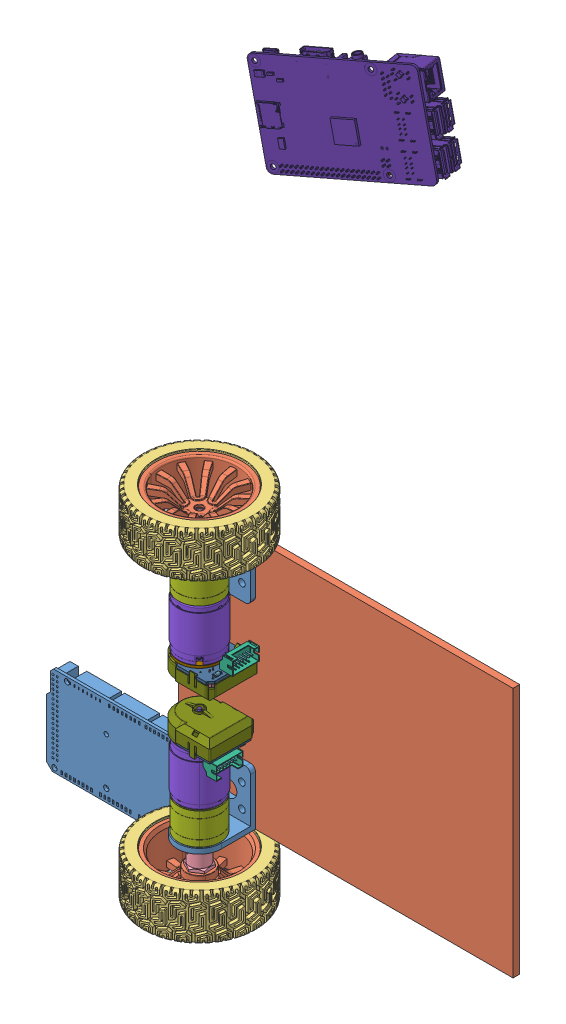
SolidWorks assembly Assem, configuration Default. Lengths in mm.
Overall size (317.13 492.65 120.83).
79 component instances, 20 part files, 16 mates.
Components (placement in the parent):
- GA25-Motor-Bracket-1: GA25-Motor-Bracket [Default] at (25.6332 -111.1645 34.9794) size (26.2 32.8 33.5)
- 65mm tire.STEP-1: 65mm tire.STEP [Default] at (58.9072 82.7048 47.6784) x (0 1 0) z (-0.275321 0 0.961352) size (31.76 86.61 86.6)
  - ________.STEP-1: ________.STEP [Default] x (1 0 0) z (0 0.808864 0.587995) size (25 51.5 51.5)
  - ____.STEP-1: ____.STEP [Default] x (1 0 0) z (0 0.328458 0.944518) size (27.02 68.04 68.02)
  - 3MM______.STEP-1: 3MM______.STEP [Default] x (0 0.808864 0.587995) z (-1 0 0) size (13.83 12.01 18.25)
- JGA25-371_ASM_Motor.STEP-1: JGA25-371_ASM_Motor.STEP [Default] at (77.6364 17.4149 55.4313) x (0.707107 0 -0.707107) z (0 1 0) size (46.57 45.86 75)
  - Socket_ASM_Varsay_lan.STEP-1: Socket_ASM_Varsay_lan.STEP [Default] at (11.1968 13.0195 -8.032) x (0.707107 -0.707107 0) z (-0.707107 -0.707107 0) size (8 10.5 16)
    - pin_Varsay_lan.STEP-1: pin_Varsay_lan.STEP [Default] at (-1.4404 -2.228 9.4706) size (6.3 6.8 0.6)
    - Socket_body_Varsay_lan.STEP-1: Socket_body_Varsay_lan.STEP [Default] at (-2.4404 0.272 12.4706) x (0 0 -1) z (1 0 0) size (16 8 8)
    - pin_Varsay_lan.STEP-2: pin_Varsay_lan.STEP [Default] at (-1.4404 -2.228 7.4706) size (6.3 6.8 0.6)
    - pin_Varsay_lan.STEP-3: pin_Varsay_lan.STEP [Default] at (-1.4404 -2.228 5.4706) size (6.3 6.8 0.6)
    - pin_Varsay_lan.STEP-4: pin_Varsay_lan.STEP [Default] at (-1.4404 -2.228 3.4706) size (6.3 6.8 0.6)
    - pin_Varsay_lan.STEP-5: pin_Varsay_lan.STEP [Default] at (-1.4404 -2.228 1.4706) size (6.3 6.8 0.6)
    - pin_Varsay_lan.STEP-6: pin_Varsay_lan.STEP [Default] at (-1.4404 -2.228 -0.5294) size (6.3 6.8 0.6)
  - Gear_box_Varsay_lan.STEP-1: Gear_box_Varsay_lan.STEP [Default] at (-7.7614 18.7257 24.5399) size (25 25 30.5)
  - Mitsumi M25N-2R-14_Varsay_lan.STEP-1: Mitsumi M25N-2R-14_Varsay_lan.STEP [Default] at (-7.7614 18.7257 -4.2601) size (25.8 25.7 54)
  - PCB1_Varsay_lan.STEP-1: PCB1_Varsay_lan.STEP [Default] at (-7.7614 18.7257 -7.7601) size (24.8 24.8 1.5)
  - PCB2_Varsay_lan.STEP-1: PCB2_Varsay_lan.STEP [Default] at (-7.7614 18.7257 -7.7601) x (-0.707107 -0.707107 0) z (0 0 -1) size (27.8 35.55 1.5)
  - Washer_Varsay_lan.STEP-1: Washer_Varsay_lan.STEP [Default] at (-7.7614 18.7257 -11.9601) size (8 8 4)
  - Encoder_disk_Varsay_lan.STEP-1: Encoder_disk_Varsay_lan.STEP [Default] at (-7.7614 18.7257 -13.4601) size (22 22 2.5)
  - Sensor_cover_Varsay_lan.STEP-1: Sensor_cover_Varsay_lan.STEP [Default] at (1.5017 4.6542 -9.2601) x (-0.707107 -0.707107 0) z (0 0 -1) size (6 14 10.5)
  - Resistor_Varsay_lan.STEP-1: Resistor_Varsay_lan.STEP [Default] at (-2.0338 -1.0026 -10.2601) x (0.707107 -0.707107 0) z (-0.707107 -0.707107 0) size (2 4.5 5.6)
  - Solder_Varsay_lan.STEP-1: Solder_Varsay_lan.STEP [Default] at (-2.0338 -1.0026 -9.2601) x (-0.923728 -0.383049 0) z (0 0 -1) size (1 1 0.9)
  - Solder_Varsay_lan.STEP-2: Solder_Varsay_lan.STEP [Default] at (1.5017 2.5329 -9.2601) x (-0.923728 -0.383049 0) z (0 0 -1) size (1 1 0.9)
  - Solder_Varsay_lan.STEP-3: Solder_Varsay_lan.STEP [Default] at (10.5527 14.4123 -9.2601) x (-0.923728 -0.383049 0) z (0 0 -1) size (1 1 0.9)
  - Solder_Varsay_lan.STEP-4: Solder_Varsay_lan.STEP [Default] at (9.1384 12.9981 -9.2601) x (-0.923728 -0.383049 0) z (0 0 -1) size (1 1 0.9)
  - Solder_Varsay_lan.STEP-5: Solder_Varsay_lan.STEP [Default] at (7.7242 11.5839 -9.2601) x (-0.923728 -0.383049 0) z (0 0 -1) size (1 1 0.9)
  - Solder_Varsay_lan.STEP-6: Solder_Varsay_lan.STEP [Default] at (6.31 10.1697 -9.2601) x (-0.923728 -0.383049 0) z (0 0 -1) size (1 1 0.9)
  - Solder_Varsay_lan.STEP-7: Solder_Varsay_lan.STEP [Default] at (4.8958 8.7555 -9.2601) x (-0.923728 -0.383049 0) z (0 0 -1) size (1 1 0.9)
  - Solder_Varsay_lan.STEP-8: Solder_Varsay_lan.STEP [Default] at (3.4816 7.3413 -9.2601) x (-0.923728 -0.383049 0) z (0 0 -1) size (1 1 0.9)
  - Solder_Varsay_lan.STEP-9: Solder_Varsay_lan.STEP [Default] at (11.9669 12.9981 -9.2601) x (-0.923728 -0.383049 0) z (0 0 -1) size (1 1 0.9)
  - Solder_Varsay_lan.STEP-10: Solder_Varsay_lan.STEP [Default] at (10.5527 11.5839 -9.2601) x (-0.923728 -0.383049 0) z (0 0 -1) size (1 1 0.9)
  - Solder_Varsay_lan.STEP-11: Solder_Varsay_lan.STEP [Default] at (9.1384 10.1697 -9.2601) x (-0.923728 -0.383049 0) z (0 0 -1) size (1 1 0.9)
  - Solder_Varsay_lan.STEP-12: Solder_Varsay_lan.STEP [Default] at (7.7242 8.7555 -9.2601) x (-0.923728 -0.383049 0) z (0 0 -1) size (1 1 0.9)
  - Solder_Varsay_lan.STEP-13: Solder_Varsay_lan.STEP [Default] at (6.31 7.3413 -9.2601) x (-0.923728 -0.383049 0) z (0 0 -1) size (1 1 0.9)
  - Solder_Varsay_lan.STEP-14: Solder_Varsay_lan.STEP [Default] at (4.8958 5.927 -9.2601) x (-0.923728 -0.383049 0) z (0 0 -1) size (1 1 0.9)
  - Encoder_case_Varsay_lan.STEP-1: Encoder_case_Varsay_lan.STEP [Default] at (-7.7614 18.7257 -9.2601) x (-0.707107 -0.707107 0) z (0 0 -1) size (28.8 36.06 13.7)
- JGA25-371_ASM_Motor.STEP-2: JGA25-371_ASM_Motor.STEP [Default] at (77.6364 -39.5052 39.9255) x (0.707107 0 0.707107) z (0 -1 0) size (46.57 45.86 75)
  - Socket_ASM_Varsay_lan.STEP-1: Socket_ASM_Varsay_lan.STEP [Default] at (11.1968 13.0195 -8.032) x (0.707107 -0.707107 0) z (-0.707107 -0.707107 0) size (8 10.5 16)
    - pin_Varsay_lan.STEP-1: pin_Varsay_lan.STEP [Default] at (-1.4404 -2.228 9.4706) size (6.3 6.8 0.6)
    - Socket_body_Varsay_lan.STEP-1: Socket_body_Varsay_lan.STEP [Default] at (-2.4404 0.272 12.4706) x (0 0 -1) z (1 0 0) size (16 8 8)
    - pin_Varsay_lan.STEP-2: pin_Varsay_lan.STEP [Default] at (-1.4404 -2.228 7.4706) size (6.3 6.8 0.6)
    - pin_Varsay_lan.STEP-3: pin_Varsay_lan.STEP [Default] at (-1.4404 -2.228 5.4706) size (6.3 6.8 0.6)
    - pin_Varsay_lan.STEP-4: pin_Varsay_lan.STEP [Default] at (-1.4404 -2.228 3.4706) size (6.3 6.8 0.6)
    - pin_Varsay_lan.STEP-5: pin_Varsay_lan.STEP [Default] at (-1.4404 -2.228 1.4706) size (6.3 6.8 0.6)
    - pin_Varsay_lan.STEP-6: pin_Varsay_lan.STEP [Default] at (-1.4404 -2.228 -0.5294) size (6.3 6.8 0.6)
  - Gear_box_Varsay_lan.STEP-1: Gear_box_Varsay_lan.STEP [Default] at (-7.7614 18.7257 24.5399) size (25 25 30.5)
  - Mitsumi M25N-2R-14_Varsay_lan.STEP-1: Mitsumi M25N-2R-14_Varsay_lan.STEP [Default] at (-7.7614 18.7257 -4.2601) size (25.8 25.7 54)
  - PCB1_Varsay_lan.STEP-1: PCB1_Varsay_lan.STEP [Default] at (-7.7614 18.7257 -7.7601) size (24.8 24.8 1.5)
  - PCB2_Varsay_lan.STEP-1: PCB2_Varsay_lan.STEP [Default] at (-7.7614 18.7257 -7.7601) x (-0.707107 -0.707107 0) z (0 0 -1) size (27.8 35.55 1.5)
  - Washer_Varsay_lan.STEP-1: Washer_Varsay_lan.STEP [Default] at (-7.7614 18.7257 -11.9601) size (8 8 4)
  - Encoder_disk_Varsay_lan.STEP-1: Encoder_disk_Varsay_lan.STEP [Default] at (-7.7614 18.7257 -13.4601) size (22 22 2.5)
  - Sensor_cover_Varsay_lan.STEP-1: Sensor_cover_Varsay_lan.STEP [Default] at (1.5017 4.6542 -9.2601) x (-0.707107 -0.707107 0) z (0 0 -1) size (6 14 10.5)
  - Resistor_Varsay_lan.STEP-1: Resistor_Varsay_lan.STEP [Default] at (-2.0338 -1.0026 -10.2601) x (0.707107 -0.707107 0) z (-0.707107 -0.707107 0) size (2 4.5 5.6)
  - Solder_Varsay_lan.STEP-1: Solder_Varsay_lan.STEP [Default] at (-2.0338 -1.0026 -9.2601) x (-0.923728 -0.383049 0) z (0 0 -1) size (1 1 0.9)
  - Solder_Varsay_lan.STEP-2: Solder_Varsay_lan.STEP [Default] at (1.5017 2.5329 -9.2601) x (-0.923728 -0.383049 0) z (0 0 -1) size (1 1 0.9)
  - Solder_Varsay_lan.STEP-3: Solder_Varsay_lan.STEP [Default] at (10.5527 14.4123 -9.2601) x (-0.923728 -0.383049 0) z (0 0 -1) size (1 1 0.9)
  - Solder_Varsay_lan.STEP-4: Solder_Varsay_lan.STEP [Default] at (9.1384 12.9981 -9.2601) x (-0.923728 -0.383049 0) z (0 0 -1) size (1 1 0.9)
  - Solder_Varsay_lan.STEP-5: Solder_Varsay_lan.STEP [Default] at (7.7242 11.5839 -9.2601) x (-0.923728 -0.383049 0) z (0 0 -1) size (1 1 0.9)
  - Solder_Varsay_lan.STEP-6: Solder_Varsay_lan.STEP [Default] at (6.31 10.1697 -9.2601) x (-0.923728 -0.383049 0) z (0 0 -1) size (1 1 0.9)
  - Solder_Varsay_lan.STEP-7: Solder_Varsay_lan.STEP [Default] at (4.8958 8.7555 -9.2601) x (-0.923728 -0.383049 0) z (0 0 -1) size (1 1 0.9)
  - Solder_Varsay_lan.STEP-8: Solder_Varsay_lan.STEP [Default] at (3.4816 7.3413 -9.2601) x (-0.923728 -0.383049 0) z (0 0 -1) size (1 1 0.9)
  - Solder_Varsay_lan.STEP-9: Solder_Varsay_lan.STEP [Default] at (11.9669 12.9981 -9.2601) x (-0.923728 -0.383049 0) z (0 0 -1) size (1 1 0.9)
  - Solder_Varsay_lan.STEP-10: Solder_Varsay_lan.STEP [Default] at (10.5527 11.5839 -9.2601) x (-0.923728 -0.383049 0) z (0 0 -1) size (1 1 0.9)
  - Solder_Varsay_lan.STEP-11: Solder_Varsay_lan.STEP [Default] at (9.1384 10.1697 -9.2601) x (-0.923728 -0.383049 0) z (0 0 -1) size (1 1 0.9)
  - Solder_Varsay_lan.STEP-12: Solder_Varsay_lan.STEP [Default] at (7.7242 8.7555 -9.2601) x (-0.923728 -0.383049 0) z (0 0 -1) size (1 1 0.9)
  - Solder_Varsay_lan.STEP-13: Solder_Varsay_lan.STEP [Default] at (6.31 7.3413 -9.2601) x (-0.923728 -0.383049 0) z (0 0 -1) size (1 1 0.9)
  - Solder_Varsay_lan.STEP-14: Solder_Varsay_lan.STEP [Default] at (4.8958 5.927 -9.2601) x (-0.923728 -0.383049 0) z (0 0 -1) size (1 1 0.9)
  - Encoder_case_Varsay_lan.STEP-1: Encoder_case_Varsay_lan.STEP [Default] at (-7.7614 18.7257 -9.2601) x (-0.707107 -0.707107 0) z (0 0 -1) size (28.8 36.06 13.7)
- 65mm tire.STEP-2: 65mm tire.STEP [Default] at (58.9072 -104.7952 47.6784) x (0 -1 0) z (-0.162875 0 -0.986647) size (31.76 86.61 86.6)
  - ________.STEP-1: ________.STEP [Default] x (1 0 0) z (0 0.808864 0.587995) size (25 51.5 51.5)
  - ____.STEP-1: ____.STEP [Default] x (1 0 0) z (0 0.328458 0.944518) size (27.02 68.04 68.02)
  - 3MM______.STEP-1: 3MM______.STEP [Default] x (0 0.808864 0.587995) z (-1 0 0) size (13.83 12.01 18.25)
- GA25-Motor-Bracket-2: GA25-Motor-Bracket [Default] at (92.1812 89.0741 34.9794) x (-1 0 0) z (0 0 1) size (26.2 32.8 33.5)
- RASPBERRY PI 3 + Female Header.STEP-1: RASPBERRY PI 3 + Female Header.STEP [Default] at (113.6624 297.3087 17.1933) x (0.929305 0.25267 -0.269352) z (-0.274831 0.960326 -0.047358) size (87.8 19.8 58)
  - RASPBERRY PI 3 MODEL B---3DModel-STEP-56544.STEP-1: RASPBERRY PI 3 MODEL B---3DModel-STEP-56544.STEP [Default] at origin size (87.8 19.8 58)
  - 40-Pin Header - Female - Double - 2.54mm.STEP-1: 40-Pin Header - Female - Double - 2.54mm.STEP [Default] at (-34.13 12.286 -25.75) x (1 0 0) z (0 -1 0) size (51.3 5 11.5)
- ArduinoMega-1: ArduinoMega [Default] at (-40.3003 -128.1419 -12.3817) size (107.95 53.42 12.95)
- BOdy-1: BOdy [Default] at (126.0335 -11.0452 23.2784) x (1 0 0) z (0 -1 0) size (200 4 150)
Mates (geometry in assembly coordinates):
- Concentric1: concentric anti-aligned: cylinder of 65mm tire.STEP-1/3MM______.STEP-1 through (58.9072 82.7048 47.6784) axis (0 1 0) radius 5.75; cylinder of JGA25-371_ASM_Motor.STEP-1/Gear_box_Varsay_lan.STEP-1 through (58.9072 72.4548 47.6784) axis (0 -1 0) radius 2
- Concentric4: concentric anti-aligned: cylinder of GA25-Motor-Bracket-1 through (58.9072 60.9548 47.6784) axis (0 -1 0) radius 4; cylinder of 65mm tire.STEP-1/3MM______.STEP-1 through (58.9072 82.7048 47.6784) axis (0 1 0) radius 5.75
- Coincident5: coincident anti-aligned: plane of GA25-Motor-Bracket-1 through (58.9072 60.9548 47.6784) normal (0 -1 0); plane of JGA25-371_ASM_Motor.STEP-1/Gear_box_Varsay_lan.STEP-1 through (58.9072 60.9548 47.6784) normal (0 1 0)
- Coincident6: coincident anti-aligned: plane of 65mm tire.STEP-1/3MM______.STEP-1 through (52.5067 64.4548 50.0123) normal (0 -1 0); plane of JGA25-371_ASM_Motor.STEP-1/Gear_box_Varsay_lan.STEP-1 through (58.9072 64.4548 47.6784) normal (0 1 0)
- Parallel1: parallel aligned: line of GA25-Motor-Bracket-1 through (69.0072 31.1548 27.2784) axis (-1 0 0); line of JGA25-371_ASM_Motor.STEP-1/Encoder_case_Varsay_lan.STEP-1 through (78.6572 1.6548 33.2784) axis (-1 0 0)
- Concentric5: concentric anti-aligned: cylinder of 65mm tire.STEP-2/3MM______.STEP-1 through (58.9072 -104.7952 47.6784) axis (0 -1 0) radius 5.75; cylinder of GA25-Motor-Bracket-2 through (58.9072 -83.0452 47.6784) axis (0 1 0) radius 4
- Coincident8: coincident anti-aligned: plane of JGA25-371_ASM_Motor.STEP-2/Gear_box_Varsay_lan.STEP-1 through (58.9072 -83.0452 47.6784) normal (0 -1 0); plane of GA25-Motor-Bracket-2 through (58.9072 -83.0452 47.6784) normal (0 1 0)
- Coincident9: coincident anti-aligned: plane of JGA25-371_ASM_Motor.STEP-2/Gear_box_Varsay_lan.STEP-1 through (58.9072 -86.5452 47.6784) normal (0 -1 0); plane of 65mm tire.STEP-2/3MM______.STEP-1 through (52.8178 -86.5452 44.6236) normal (0 1 0)
- Concentric6: concentric anti-aligned: cylinder of JGA25-371_ASM_Motor.STEP-2/Gear_box_Varsay_lan.STEP-1 through (58.9072 -94.5452 47.6784) axis (0 1 0) radius 2; cylinder of 65mm tire.STEP-2/3MM______.STEP-1 through (58.9072 -104.7952 47.6784) axis (0 -1 0) radius 5.75
- Coincident10: coincident aligned: plane of GA25-Motor-Bracket-1 through (58.9072 47.5548 27.2784) normal (0 0 -1); plane of GA25-Motor-Bracket-2 through (58.9072 -69.6452 27.2784) normal (0 0 -1)
- Coincident11: coincident aligned: line of GA25-Motor-Bracket-1 through (45.8072 34.1548 27.2784) axis (0 1 0); line of GA25-Motor-Bracket-2 through (45.8072 -86.0452 27.2784) axis (0 1 0)
- Parallel3: parallel aligned: line of JGA25-371_ASM_Motor.STEP-2/Encoder_case_Varsay_lan.STEP-1 through (59.1572 -23.7452 33.2784) axis (1 0 0); line of GA25-Motor-Bracket-2 through (48.8072 -53.2452 27.2784) axis (1 0 0)
- Distance3: distance = 150 mm: line of GA25-Motor-Bracket-2 through (72.0072 -86.0452 27.2784) axis (-1 0 0); line of GA25-Motor-Bracket-1 through (45.8072 63.9548 27.2784) axis (1 0 0)
- Coincident12: coincident: plane of GA25-Motor-Bracket-1 through (58.9072 47.5548 27.2784) normal (0 0 -1); plane of BOdy-1 through (100.1582 -11.0452 27.2784) normal (0 0 1)
- Coincident14: coincident: line of GA25-Motor-Bracket-1 through (45.8072 63.9548 27.2784) axis (1 0 0); line of BOdy-1 through (200.1582 63.9548 27.2784) axis (-1 0 0)
- Distance4: distance = 20 mm: line of GA25-Motor-Bracket-2 through (45.8072 -56.2452 30.2784) axis (0 -1 0); line of BOdy-1 through (26.0335 63.9548 27.2784) axis (0 -1 0)
